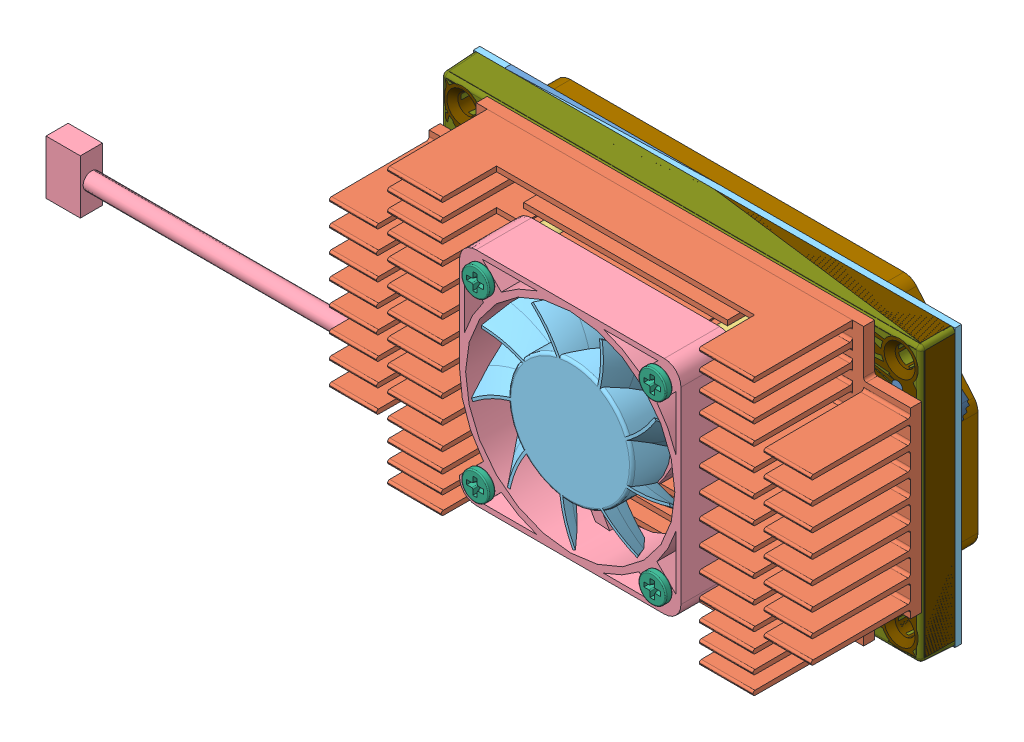
SolidWorks assembly JETSON-NEW_ASM, configuration Default. Lengths in mm. (continued)
Components (placement in the parent): (continued)
- 244-82180-1000-A03-10-12-15_ASM-1: 244-82180-1000-A03-10-12-15_ASM [Default] at origin size (87 50 8.3) (continued)
  - 100-0063-000_1-7: 100-0063-000_1 [Default] at (33.943 9.709 1.164) x (0 -1 0) z (0 0 1) size (1.75 0.53 0.55)
  - 100-0189-000_2-1: 100-0189-000_2 [Default] at (43.113 20.934 0) x (1 0 0) z (0 0 -1) size (1.75 0.53 0.55)
  - 100-0063-000_1-8: 100-0063-000_1 [Default] at (46.76 10.216 1.164) size (1.75 0.53 0.55)
  - 100-0189-000_2-2: 100-0189-000_2 [Default] at (22.95 25.35 1.164) x (-1 0 0) z (0 0 1) size (1.75 0.53 0.55)
  - 100-0063-000_1-9: 100-0063-000_1 [Default] at (46.93 23.266 1.164) size (1.75 0.53 0.55)
  - 100-0165-000_1-1: 100-0165-000_1 [Default] at (73.7 12.5 0) x (0 -1 0) z (0 0 -1) size (1.75 0.53 0.6)
  - 195-1592-000_1-1: 195-1592-000_1 [Default] at (55.8 11.95 0) x (1 0 0) z (0 0 -1) size (3.05 1.27 0.65)
  - 195-1592-000_1-2: 195-1592-000_1 [Default] at (60.75 14.4 0) x (0 -1 0) z (0 0 -1) size (3.05 1.27 0.65)
  - 039-0122-000_1-1: 039-0122-000_1 [Default] at (53.84 22.3 0) x (0 -1 0) z (0 0 -1) size (3.05 1.27 0.95)
  - 039-0122-000_1-2: 039-0122-000_1 [Default] at (55.93 22.35 0) x (0 -1 0) z (0 0 -1) size (3.05 1.27 0.95)
  - 032-0037-000_2-1: 032-0037-000_2 [Default] at (47.8 13.8 0) x (1 0 0) z (0 0 -1) size (3.05 1.27 0.95)
  - 032-0037-000_2-2: 032-0037-000_2 [Default] at (40.15 26.75 0) x (1 0 0) z (0 0 -1) size (3.05 1.27 0.95)
  - 039-0122-000_1-3: 039-0122-000_1 [Default] at (47.153 31.164 0) x (0 1 0) z (0 0 -1) size (3.05 1.27 0.95)
  - 039-0122-000_1-4: 039-0122-000_1 [Default] at (48.803 31.154 0) x (0 1 0) z (0 0 -1) size (3.05 1.27 0.95)
  - 039-0122-000_1-5: 039-0122-000_1 [Default] at (47.278 13.804 1.164) x (0 -1 0) z (0 0 1) size (3.05 1.27 0.95)
  - 032-0037-000_2-3: 032-0037-000_2 [Default] at (47.778 15.548 0) x (1 0 0) z (0 0 -1) size (3.05 1.27 0.95)
  - 032-0037-000_2-4: 032-0037-000_2 [Default] at (48.978 13.804 1.164) x (0 -1 0) z (0 0 1) size (3.05 1.27 0.95)
  - 039-0122-000_1-6: 039-0122-000_1 [Default] at (49.67 20.36 0) x (1 0 0) z (0 0 -1) size (3.05 1.27 0.95)
  - 032-0037-000_2-5: 032-0037-000_2 [Default] at (47.778 17.15 0) x (1 0 0) z (0 0 -1) size (3.05 1.27 0.95)
  - 032-0037-000_2-6: 032-0037-000_2 [Default] at (50.678 13.804 1.164) x (0 -1 0) z (0 0 1) size (3.05 1.27 0.95)
  - 039-0122-000_1-7: 039-0122-000_1 [Default] at (59.544 23.53 0) x (1 0 0) z (0 0 -1) size (3.05 1.27 0.95)
  - 039-0122-000_1-8: 039-0122-000_1 [Default] at (57.95 28.15 1.164) size (3.05 1.27 0.95)
  - 039-0122-000_1-9: 039-0122-000_1 [Default] at (59.515 25.132 0) x (1 0 0) z (0 0 -1) size (3.05 1.27 0.95)
  - 039-0122-000_1-10: 039-0122-000_1 [Default] at (59.483 28.504 0) x (1 0 0) z (0 0 -1) size (3.05 1.27 0.95)
  - 039-0122-000_1-11: 039-0122-000_1 [Default] at (59.483 26.754 0) x (1 0 0) z (0 0 -1) size (3.05 1.27 0.95)
  - 039-0122-000_1-12: 039-0122-000_1 [Default] at (59.483 30.134 0) x (1 0 0) z (0 0 -1) size (3.05 1.27 0.95)
  - 215-0165-000_1-1: 215-0165-000_1 [Default] at (74.133 26.474 1.164) size (3.05 1.27 0.6)
  - 215-0165-000_1-2: 215-0165-000_1 [Default] at (74.004 19.097 1.164) x (0 1 0) z (0 0 1) size (3.05 1.27 0.6)
  - 039-0190-000_1-1: 039-0190-000_1 [Default] at (62.5 12.45 0) x (0 -1 0) z (0 0 -1) size (3.05 1.27 0.95)
  - 100-0077-000_1-1: 100-0077-000_1 [Default] at (16.393 37.444 1.164) x (-1 0 0) z (0 0 1) size (2.22 0.81 0.95)
  - 085-0232-000_1-1: 085-0232-000_1 [Default] at (66.12 7.63 1.164) x (-1 0 0) z (0 0 1) size (3.81 2.5 0.75)
  - 161-0188-600_2_GREY-1: 161-0188-600_2_GREY [Default] at (28.903 37.199 1.164) x (0 1 0) z (0 0 1) size (10.1 15.1 1)
  - 161-0188-600_2_GREY-2: 161-0188-600_2_GREY [Default] at (44.603 37.199 1.164) x (0 1 0) z (0 0 1) size (10.1 15.1 1)
  - 300-0868-000_3-1: 300-0868-000_3 [Default] at (53.3 9.55 1.164) size (1 0.6 0.41)
  - 300-0868-000_3-2: 300-0868-000_3 [Default] at (15.5 12.85 0) x (-1 0 0) z (0 0 -1) size (1 0.6 0.41)
  - 300-0868-000_3-3: 300-0868-000_3 [Default] at (71 25.95 0) x (1 0 0) z (0 0 -1) size (1 0.6 0.41)
  - 300-0868-000_3-4: 300-0868-000_3 [Default] at (63.55 39 0) x (1 0 0) z (0 0 -1) size (1 0.6 0.41)
  - 300-0870-000_1-1: 300-0870-000_1 [Default] at (31.482 11.077 0) x (-1 0 0) z (0 0 -1) size (1 0.6 0.41)
  - 131-0632-000_2-1: 131-0632-000_2 [Default] at (72.11 12.9 1.164) size (3.05 1.27 1.4)
  - 300-0494-000_1-1: 300-0494-000_1 [Default] at (71.55 15.75 0) x (1 0 0) z (0 0 -1) size (2.94 3.2 1.21)
  - 080-0550-000_2-1: 080-0550-000_2 [Default] at (-1.294 28.232 1.164) x (0 1 0) z (0 0 1) size (3.63 4.07 1.47)
  - 080-0550-000_2-2: 080-0550-000_2 [Default] at (-1.294 33.789 1.164) x (0 1 0) z (0 0 1) size (3.63 4.07 1.47)
- 320-1117-000-1: 320-1117-000 [Default] at (1.45 38.9 2.5402) x (0 -1 0) z (-1 0 0) size (12.27 1.42 18.87)
- 285-0185-000-1: 285-0185-000 [Default] at (32.053 14.304 2.164) size (9 9 0.01)
- 285-0146-000-1: 285-0146-000 [Default] at (21.203 32.699 2.164) size (31 9 0.01)
- 285-0091-000-CG-1: 285-0091-000-CG [Default] at (4.6 13.9 1.809) size (12 10 0.01)
- 285-0181-000-1: 285-0181-000 [Default] at (64.584 31.59 3.0403) size (6 6 0.01)
- TTP-1_ASM-1: TTP-1_ASM [Default] at (-4 -4 1.164) size (87 50 7.36)
  - TTP-1: TTP [Default] at origin size (87 50 6.16)
  - PIN-DOWEL-1MM-1: PIN-DOWEL-1MM [Default] at (4.432 8.418 6) x (1 0 0) z (0 1 0) size (2 7.2 2)
  - PIN-DOWEL-1MM-2: PIN-DOWEL-1MM [Default] at (82.57 41.58 6) x (1 0 0) z (0 1 0) size (2 7.2 2)
- TTP-1-REV5-2015-0727_ASM-1: TTP-1-REV5-2015-0727_ASM [Default] at (-4 -4 1.164) size (87.01 50.01 7.22)
  - TTP-1-REV5_ASM_6_ASM-1: TTP-1-REV5_ASM_6_ASM [Default] at origin size (87.01 50.01 7.22)
    - TTP_1-REV5_31-1: TTP_1-REV5_31 [Default] at origin size (87.01 50.01 6.07)
    - PIN-DOWEL-1MM_1_1-1: PIN-DOWEL-1MM_1_1 [Default] at (4.432 8.418 6) x (1 0 0) z (0 1 0) size (2 7.2 2)
    - PIN-DOWEL-1MM_1_1-2: PIN-DOWEL-1MM_1_1 [Default] at (82.57 41.58 6) x (1 0 0) z (0 1 0) size (2 7.2 2)
- DCV-01672-N1-GP-08-12-15_ASM-1: DCV-01672-N1-GP-08-12-15_ASM [Default] at (83 46 7.164) x (-1 0 0) z (0 0 1) size (144.7 50 21.24)
  - JETSON-DEV-COOLER_ASM_5_ASM-1: JETSON-DEV-COOLER_ASM_5_ASM [Default] at origin size (144.7 50 21.24)
    - DEV-HEATSINK-2015-0717_ASM_3_ASM-1: DEV-HEATSINK-2015-0717_ASM_3_ASM [Default] at origin size (87 50 20)
      - DEV-HS-VO_6-1: DEV-HS-VO_6 [Default] at origin size (87 50 20)
      - STANDOFF_3_1-1: STANDOFF_3_1 [Default] at (59.5 9 0.1) x (-1 0 0) z (0 1 0) size (5.5 9.9 5.5)
      - STANDOFF_3_1-2: STANDOFF_3_1 [Default] at (59.5 41 0.1) x (-1 0 0) z (0 1 0) size (5.5 9.9 5.5)
      - STANDOFF_3_1-3: STANDOFF_3_1 [Default] at (27.5 41 0.1) x (-1 0 0) z (0 1 0) size (5.5 9.9 5.5)
      - STANDOFF_3_1-4: STANDOFF_3_1 [Default] at (27.5 9 0.1) x (-1 0 0) z (0 1 0) size (5.5 9.9 5.5)
    - FANKUANG_0104-1: FANKUANG_0104 [Default] at (43.5 25 10) x (1 0 0) z (0 -1 0) size (121.2 10.5 40)
    - FANYE_0104-1: FANYE_0104 [Default] at (43.5 25 13) x (-1 0 0) z (0 1 0) size (36.31 7.05 36.51)
    - FAN-SCREW-M2-L15-2_1-1: FAN-SCREW-M2-L15-2_1 [Default] at (59.5 41 20) x (-1 0 0) z (0 0 -1) size (5 5 15.41)
    - FAN-SCREW-M2-L15-2_1-2: FAN-SCREW-M2-L15-2_1 [Default] at (59.5 9 20) x (-1 0 0) z (0 0 -1) size (5 5 15.41)
    - FAN-SCREW-M2-L15-2_1-3: FAN-SCREW-M2-L15-2_1 [Default] at (27.5 41 20) x (-1 0 0) z (0 0 -1) size (5 5 15.41)
    - FAN-SCREW-M2-L15-2_1-4: FAN-SCREW-M2-L15-2_1 [Default] at (27.5 9 20) x (-1 0 0) z (0 0 -1) size (5 5 15.41)
    - GREASE-X23-7762_2-1: GREASE-X23-7762_2 [Default] at origin size (42 26 0.2)
- 155-0096-000-1: 155-0096-000 [Default] at (18.64 0.14 9.164) x (-1 0 0) z (0 1 0) size (3.99 5.65 3.99)
- 155-0096-000-2: 155-0096-000 [Default] at (60.36 0.14 9.164) x (-1 0 0) z (0 1 0) size (3.99 5.65 3.99)
- 155-0096-000-3: 155-0096-000 [Default] at (18.64 41.86 9.164) x (-1 0 0) z (0 1 0) size (3.99 5.65 3.99)
- 155-0096-000-4: 155-0096-000 [Default] at (60.36 41.86 9.164) x (-1 0 0) z (0 1 0) size (3.99 5.65 3.99)
- JETSON-BOTTOM-COVER-1: JETSON-BOTTOM-COVER [Default] at (83 8.88 0) x (-1 0 0) z (0 -1 0) size (87 3 37.12)
- JETSON-BOTTOM-COVER-REV1-2015-0-1: JETSON-BOTTOM-COVER-REV1-2015-0 [Default] at (83 9 0) x (-1 0 0) z (0 -1 0) size (87 2.88 37)
- 155-0190-000-1: 155-0190-000 [Default] at (79 21 -0.9424) x (1 0 0) z (0 1 0) size (5.49 5.67 5.49)
- 155-0190-000-2: 155-0190-000 [Default] at (0 21 -0.9424) x (1 0 0) z (0 1 0) size (5.49 5.67 5.49)
